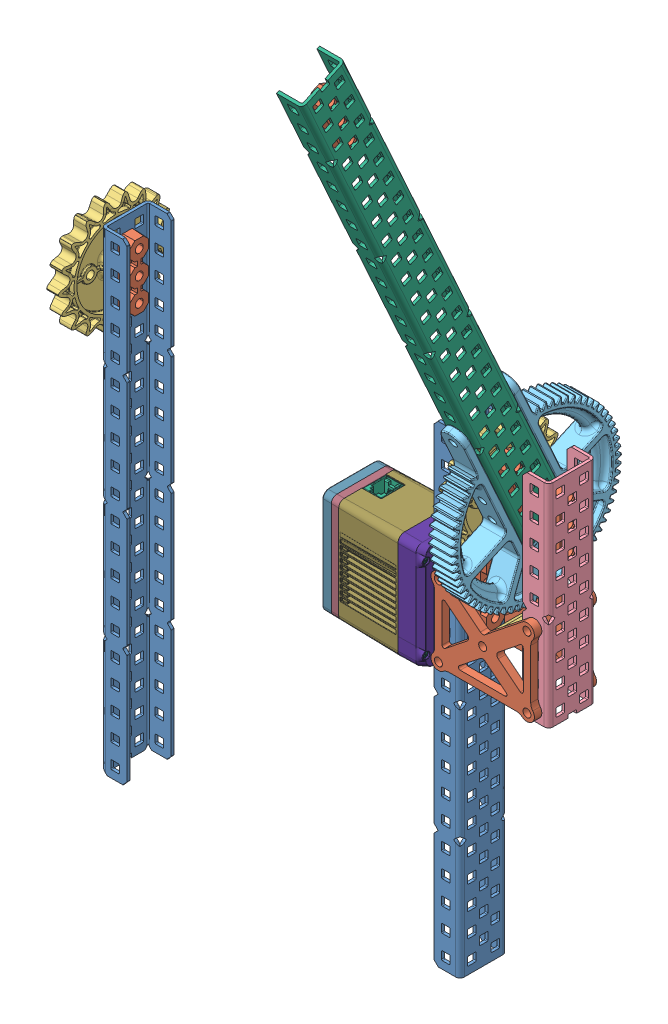
SolidWorks assembly chainbarFull, configuration Default. Lengths in mm.
Overall size (256.54 498.98 217.82).
51 component instances, 24 part files, 2 mates.
Components (placement in the parent):
- ChainbarTowers-2: ChainbarTowers [Default] at (223.5825 254.7824 221.2138) x (0 -1 0) z (-1 0 0) size (259.11 61.52 256.54)
  - 1x2x1x20 Aluminum C-Channel-1: 1x2x1x20 Aluminum C-Channel [Default] at (148.2233 92.4309 194.0391) size (254 25.41 13.97)
  - 1x2x1x20 Aluminum C-Channel-2: 1x2x1x20 Aluminum C-Channel [Default] at (-42.2767 92.4309 0.9991) x (-1 0 0) z (0 0 -1) size (254 25.41 13.97)
  - Flat Bearing (276-1209)-1: Flat Bearing (276-1209) [Default] at (-22.2107 79.7309 103.4881) x (0 0 1) z (0 -1 0) size (7.04 35.56 10.16)
  - Flat Bearing (276-1209)-2: Flat Bearing (276-1209) [Default] at (-75.0427 79.7309 91.5501) x (0 0 -1) z (0 -1 0) size (7.04 35.56 10.16)
  - 18THS_Sprocket_w_Inserts-1: 18THS_Sprocket_w_Inserts [Default] at (-67.509 55.75 -53.2065) size (61.01 61.52 15.88)
    - 18T High Strength Sprocket (HS Bore) (276-3878)-1: 18T High Strength Sprocket (HS Bore) (276-3878) [Default] at (18.8823 36.6809 46.2681) size (61.01 61.52 13.34)
    - Plastic Shaft Inserts (276-3881-001)-1: Plastic Shaft Inserts (276-3881-001) [Default] at (18.8823 36.6809 54.2056) x (1 0 0) z (0 1 0) size (10.03 5.08 10.03)
    - Plastic Shaft Inserts (276-3881-001)-2: Plastic Shaft Inserts (276-3881-001) [Default] at (18.8823 36.6809 38.3306) x (0 -1 0) z (-1 0 0) size (10.03 5.08 10.03)
  - 18THS_Sprocket_w_Inserts-2: 18THS_Sprocket_w_Inserts [Default] at (-67.509 55.75 155.7085) size (61.01 61.52 15.88)
    - 18T High Strength Sprocket (HS Bore) (276-3878)-1: 18T High Strength Sprocket (HS Bore) (276-3878) [Default] at (18.8823 36.6809 46.2681) size (61.01 61.52 13.34)
    - Plastic Shaft Inserts (276-3881-001)-1: Plastic Shaft Inserts (276-3881-001) [Default] at (18.8823 36.6809 54.2056) x (1 0 0) z (0 1 0) size (10.03 5.08 10.03)
    - Plastic Shaft Inserts (276-3881-001)-2: Plastic Shaft Inserts (276-3881-001) [Default] at (18.8823 36.6809 38.3306) x (0 -1 0) z (-1 0 0) size (10.03 5.08 10.03)
  - Flat Bearing (276-1209)-3: Flat Bearing (276-1209) [Default] at (28.5893 79.7309 -87.9771) x (0 0 1) z (0 -1 0) size (7.04 35.56 10.16)
  - V5 Smart Motor (276-4840) 2-1: V5 Smart Motor (276-4840) 2 [Default] at (14.8733 92.4309 46.7739) x (-1 0 0) z (0 0 -1) size (59.01 35.33 72.31)
    - V5 Smart Motor (276-4840) 2.step-1: V5 Smart Motor (276-4840) 2.step [Default] at origin size (59.01 35.33 72.31)
      - 276-4840-900 Rev6_Instruction.step-1: 276-4840-900 Rev6_Instruction.step [Default] at (-14.3 0 -17.2) size (52.79 15.94 38.15)
        - 276-4840-901 Rev6.step-1: 276-4840-901 Rev6.step [Default] at (10.75 -10.05 17.8) x (-1 0 0) z (0 0 1) size (49.9 1.6 38.15)
        - 276-4840-902 Rev2.step-1: 276-4840-902 Rev2.step [Default] at (31.25 -9.25 6.2) x (0 0 -1) z (0 -1 0) size (10.35 11.39 15.94)
        - 276-4840-022 Rev4.step-1: 276-4840-022 Rev4.step [Default] at (31.25 -9.25 6.2) x (0 0 -1) z (1 0 0) size (10.26 9.1 5.51)
      - 276-4840-110 Rev10_Instruction.step-1: 276-4840-110 Rev10_Instruction.step [Default] at (12.7 0 14.7) size (35.33 35.33 31.1)
        - 276-4840-061 Rev7_Ring_Gear_Fixed01 .6 Rev3.step-1: 276-4840-061 Rev7_Ring_Gear_Fixed01 .6 Rev3.step [Default] at origin size (28.79 28.39 24.6)
        - 276-4840-018 Rev6.step-1: 276-4840-018 Rev6.step [Default] at (0 0 6.7) x (-0.483174 0.875524 0) z (0 0 1) size (26 26 12.3)
        - 276-4840-059 Rev2.step-1: 276-4840-059 Rev2.step [Default] at (0 0 10.3) size (28.4 28.4 8.5)
        - 276-4840-062 Rev1.step-1: 276-4840-062 Rev1.step [Default] at (-12.1353 8.8168 12.3) x (0.956835 -0.290632 0) z (-0.290632 -0.956835 0) size (3.2 6.56 3.2)
        - 276-4840-062 Rev1.step-2: 276-4840-062 Rev1.step [Default] at (12.1353 8.8168 12.3) x (0.978427 0.206591 0) z (0.206591 -0.978427 0) size (3.2 6.56 3.2)
        - 276-4840-062 Rev1.step-3: 276-4840-062 Rev1.step [Default] at (-12.1353 -8.8168 12.3) x (0.72563 0.688086 0) z (0.688086 -0.72563 0) size (3.2 6.56 3.2)
      - 276-4840-001 Rev38.step-1: 276-4840-001 Rev38.step [Default] at origin size (57.3 33 46.9)
      - 276-4840-005 Rev27.step-1: 276-4840-005 Rev27.step [Default] at (0 0 -17.95) size (56.17 31.87 12.9)
      - 276-4840-004 Rev16.step-1: 276-4840-004 Rev16.step [Default] at (0 0 -19.2) size (56.01 31.71 9.21)
      - 276-4840-015 Rev7.step-1: 276-4840-015 Rev7.step [Default] at (-21.95 14 27.9) x (-0.85131 -0.524663 0) z (-0.524663 0.85131 0) size (3.2 17.55 3.2)
      - 276-4840-015 Rev7.step-2: 276-4840-015 Rev7.step [Default] at (21.95 -14 27.9) x (-0.777574 -0.628792 0) z (-0.628792 0.777574 0) size (3.2 17.55 3.2)
      - 276-4840-015 Rev7.step-3: 276-4840-015 Rev7.step [Default] at (21.95 14 27.9) x (0.476859 0.87898 0) z (0.87898 -0.476859 0) size (3.2 17.55 3.2)
      - 276-4840-009 Rev3.step-1: 276-4840-009 Rev3.step [Default] at (25.45 13.5 15.7) x (0.19987 -0.979823 0) z (-0.979823 -0.19987 0) size (3.4 41.31 4.34)
      - 276-4840-009 Rev3.step-2: 276-4840-009 Rev3.step [Default] at (-25.45 -13.5 15.7) x (-0.998855 0.047836 0) z (0.047836 0.998855 0) size (3.4 41.31 4.34)
      - 276-4840-009 Rev3.step-3: 276-4840-009 Rev3.step [Default] at (25.45 -13.5 15.7) x (-0.975374 0.220559 0) z (0.220559 0.975374 0) size (3.4 41.31 4.34)
      - 276-4840-009 Rev3.step-4: 276-4840-009 Rev3.step [Default] at (-25.45 13.5 15.7) x (-0.922256 0.38658 0) z (0.38658 0.922256 0) size (3.4 41.31 4.34)
      - 276-4840-003 Rev27.step-1: 276-4840-003 Rev27.step [Default] at (0 0 16.2) size (57.3 33 28.01)
      - 276-4840-043 Rev8.step-1: 276-4840-043 Rev8.step [Default] at (-12.7 0 36.2) x (-0.5 -0.866025 0) z (-0.866025 0.5 0) size (6.3 15.2 7.21)
      - 276-4840-043 Rev8.step-2: 276-4840-043 Rev8.step [Default] at (0 0 36.2) x (-0.5 -0.866025 0) z (-0.866025 0.5 0) size (6.3 15.2 7.21)
      - 276-4840-025 Rev19.step-1: 276-4840-025 Rev19.step [Default] at (12.7 0 -22.63) x (-0.993315 0.115437 0) z (0 0 1) size (14.82 14.83 35.18)
  - supportConnector-1: supportConnector [Default] at (33.9233 105.1309 8.6191) x (0 0 -1) z (0 1 0) size (55.62 46.1 4)
  - supportConnector-2: supportConnector [Default] at (33.9233 79.7309 -39.0059) x (0 0 1) z (0 -1 0) size (55.62 46.1 4)
  - 1.00_ Standoff (275-1016)-1: 1.00_ Standoff (275-1016) [Default] at (14.8733 92.4309 -15.1934) size (7.34 25.4 7.34)
  - 1x2x1x9 Aluminum C-Channel-1: 1x2x1x9 Aluminum C-Channel [Default] at (148.2233 92.4309 -46.6259) x (1 0 0) z (0 0 -1) size (113.79 25.41 13.97)
  - Flat Bearing (276-1209)-4: Flat Bearing (276-1209) [Default] at (-22.2107 105.1309 43.9251) x (0 0 -1) z (0 1 0) size (7.04 35.56 10.16)
- GearedArmAssem-1: GearedArmAssem [Default] at (213.1553 207.4979 334.4727) x (1 0 0) z (0 0.910344 0.413853) size (14.03 91.45 325.15)
  - ORION 20Pd 70T Gear (Chainbar)-1: ORION 20Pd 70T Gear (Chainbar) [Inch - Spur gear 20DP 70T 20PA 0.5FW ---S70N3.0H2.0L0.0591N] at (25.3031 58.6537 78.6924) size (12.81 91.45 109.25)
  - Flat Bearing (276-1209)-1: Flat Bearing (276-1209) [Default] at (-51.2779 71.3537 117.8084) x (1 0 0) z (0 1 0) size (7.04 35.56 10.16)
  - Flat Bearing (276-1209)-2: Flat Bearing (276-1209) [Default] at (-51.2779 45.9537 306.2764) x (1 0 0) z (0 -1 0) size (7.04 35.56 10.16)
  - 1x2x1x23 Aluminum C-Channel (276-2289)-1: 1x2x1x23 Aluminum C-Channel (276-2289) [Default] at (39.2731 58.6537 288.2424) x (0 0 1) z (1 0 0) size (292.1 25.41 13.97)
Mates (geometry in assembly coordinates):
- Concentric1: concentric aligned: cylinder of ChainbarTowers-2/18THS_Sprocket_w_Inserts-1/Plastic Shaft Inserts (276-3881-001)-2 through (238.4584 303.4091 313.6447) axis (1 0 0) radius 2.032; cylinder of GearedArmAssem-1/Flat Bearing (276-1209)-1 through (244.5036 303.4091 313.6447) axis (1 0 0) radius 2.1209
- Distance1: distance = 15.875 mm anti-aligned: plane of GearedArmAssem-1/ORION 20Pd 70T Gear (Chainbar)-1 through (238.4584 303.4091 313.6447) normal (-1 0 0); plane of ChainbarTowers-2/1x2x1x20 Aluminum C-Channel-2 through (222.5834 75.3091 291.7244) normal (1 0 0)
